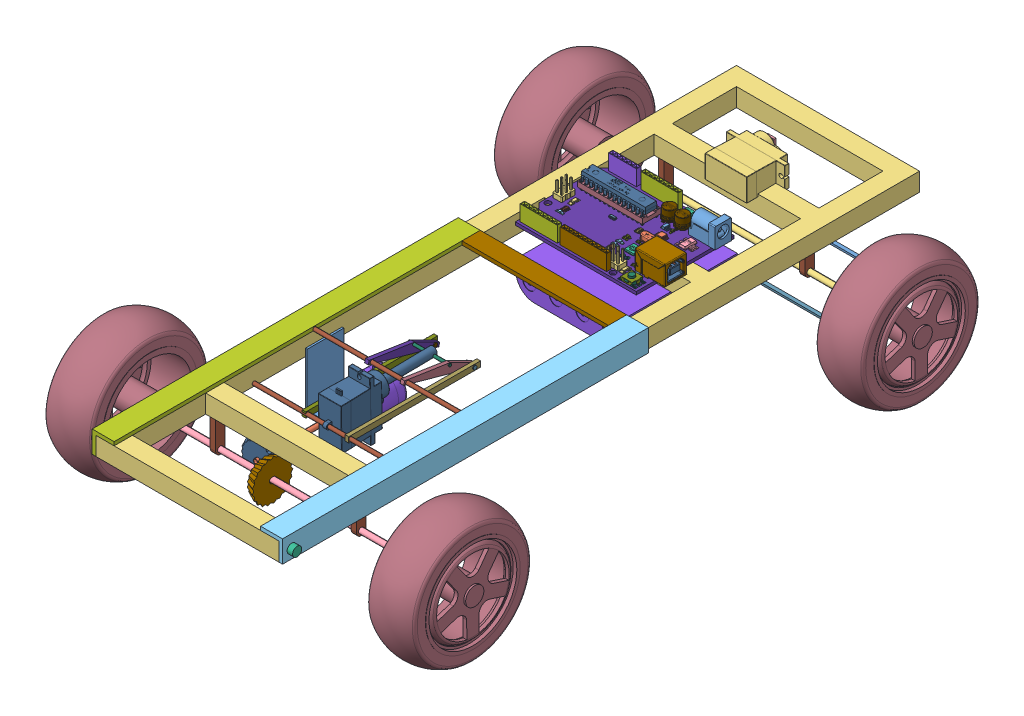
SolidWorks assembly Truck, configuration Default. Lengths in mm.
Overall size (204.96 79.96 350).
143 component instances, 76 part files, 0 mates.
Components (placement in the parent):
- truck3 v8.step-1: truck3 v8.step [Default] at origin size (204.96 79.96 350)
  - front axis.step-1: front axis.step [Default] at (0 -2.5 0) size (144 3 3)
    - Component11.step-1: Component11.step [Default] at origin size (2 2 2)
    - Component12.step-1: Component12.step [Default] at origin size (2 2 2)
    - front axis-0.step-1: front axis-0.step [Default] at origin size (140 3 3)
    - front axis-1.step-1: front axis-1.step [Default] at origin size (2 0.5 2.24)
    - front axis-2.step-1: front axis-2.step [Default] at origin size (2 0.5 2.24)
  - _Battery Holder.914559a7-a8a6-4aca-8b1f-9f589b69178d.step-1: _Battery Holder.914559a7-a8a6-4aca-8b1f-9f589b69178d.step [Default] at (0 -0.1583 -190) x (0 0 1) z (1 0 0) size (63 16 58)
    - Component1.step-1: Component1.step [Default] at origin size (13.02 9.16 9.21)
    - Component1.step-2: Component1.step [Default] at (0 0 -29) size (13.02 9.16 9.21)
    - Component2.step-1: Component2.step [Default] at origin size (13.02 9.28 9.51)
    - Component2.step-2: Component2.step [Default] at (0 0 -29) size (13.02 9.28 9.51)
    - _Battery Holder.914559a7-a8a6-4aca-8b1f-9f589b69178d-3.step-1: _Battery Holder.914559a7-a8a6-4aca-8b1f-9f589b69178d-3.step [Default] at origin size (63 16 58)
  - Arduino_uno.6df525b0-a0fc-4683-8e1a-4d70c617ad71.step-1: Arduino_uno.6df525b0-a0fc-4683-8e1a-4d70c617ad71.step [Default] at (32.62 13 -215.96) x (0 0 -1) z (1 0 0) size (53.34 15.25 74.93)
    - USB type b.step-1: USB type b.step [Default] at (-38.02 0.43 6.35) size (13.72 15.2 16.5)
      - USB SHELL.step-1: USB SHELL.step [Default] at origin size (13.72 15.2 16.5)
      - USB core.step-1: USB core.step [Default] at origin size (11.3 10.68 15.75)
      - usb top contact.step-1: usb top contact.step [Default] at (1.25 6.09 -0.38) size (1 9.67 13.76)
      - usb btm contact.step-1: usb btm contact.step [Default] at (1.25 4.41 -0.38) size (1 6.84 11.76)
      - usb btm contact.step-2: usb btm contact.step [Default] at (-1.25 4.41 -0.38) size (1 6.84 11.76)
      - usb top contact.step-2: usb top contact.step [Default] at (-1.25 6.09 -0.38) size (1 9.67 13.76)
    - dip28 (1).step-1: dip28 (1).step [Default] at (-16.383 1.5 -46.355) x (0 0 -1) z (1 0 0) size (35.48 7.37 10.1)
      - dip28.step-1: dip28.step [Default] at origin size (35.48 2.8 10.1)
      - dip socket pin.step-1: dip socket pin.step [Default] at (16.51 2.8 -3.81) size (1.7 7.37 1.7)
      - dip socket pin.step-2: dip socket pin.step [Default] at (16.51 2.8 3.81) size (1.7 7.37 1.7)
      - dip socket pin.step-3: dip socket pin.step [Default] at (13.97 2.8 -3.81) size (1.7 7.37 1.7)
      - dip socket pin.step-4: dip socket pin.step [Default] at (13.97 2.8 3.81) size (1.7 7.37 1.7)
      - dip socket pin.step-5: dip socket pin.step [Default] at (11.43 2.8 -3.81) size (1.7 7.37 1.7)
      - dip socket pin.step-6: dip socket pin.step [Default] at (11.43 2.8 3.81) size (1.7 7.37 1.7)
      - dip socket pin.step-7: dip socket pin.step [Default] at (8.89 2.8 -3.81) size (1.7 7.37 1.7)
      - dip socket pin.step-8: dip socket pin.step [Default] at (8.89 2.8 3.81) size (1.7 7.37 1.7)
      - dip socket pin.step-9: dip socket pin.step [Default] at (6.35 2.8 -3.81) size (1.7 7.37 1.7)
      - dip socket pin.step-10: dip socket pin.step [Default] at (6.35 2.8 3.81) size (1.7 7.37 1.7)
      - dip socket pin.step-11: dip socket pin.step [Default] at (3.81 2.8 -3.81) size (1.7 7.37 1.7)
      - dip socket pin.step-12: dip socket pin.step [Default] at (3.81 2.8 3.81) size (1.7 7.37 1.7)
      - dip socket pin.step-13: dip socket pin.step [Default] at (1.27 2.8 -3.81) size (1.7 7.37 1.7)
      - dip socket pin.step-14: dip socket pin.step [Default] at (1.27 2.8 3.81) size (1.7 7.37 1.7)
      - dip socket pin.step-15: dip socket pin.step [Default] at (-1.27 2.8 -3.81) size (1.7 7.37 1.7)
      - dip socket pin.step-16: dip socket pin.step [Default] at (-1.27 2.8 3.81) size (1.7 7.37 1.7)
      - dip socket pin.step-17: dip socket pin.step [Default] at (-3.81 2.8 -3.81) size (1.7 7.37 1.7)
      - dip socket pin.step-18: dip socket pin.step [Default] at (-3.81 2.8 3.81) size (1.7 7.37 1.7)
      - dip socket pin.step-19: dip socket pin.step [Default] at (-6.35 2.8 -3.81) size (1.7 7.37 1.7)
      - dip socket pin.step-20: dip socket pin.step [Default] at (-6.35 2.8 3.81) size (1.7 7.37 1.7)
      - dip socket pin.step-21: dip socket pin.step [Default] at (-8.89 2.8 -3.81) size (1.7 7.37 1.7)
      - dip socket pin.step-22: dip socket pin.step [Default] at (-8.89 2.8 3.81) size (1.7 7.37 1.7)
      - dip socket pin.step-23: dip socket pin.step [Default] at (-11.43 2.8 -3.81) size (1.7 7.37 1.7)
      - dip socket pin.step-24: dip socket pin.step [Default] at (-11.43 2.8 3.81) size (1.7 7.37 1.7)
      - dip socket pin.step-25: dip socket pin.step [Default] at (-13.97 2.8 -3.81) size (1.7 7.37 1.7)
      - dip socket pin.step-26: dip socket pin.step [Default] at (-13.97 2.8 3.81) size (1.7 7.37 1.7)
      - dip socket pin.step-27: dip socket pin.step [Default] at (-16.51 2.8 -3.81) size (1.7 7.37 1.7)
      - dip socket pin.step-28: dip socket pin.step [Default] at (-16.51 2.8 3.81) size (1.7 7.37 1.7)
    - RESET BUTTON.step-1: RESET BUTTON.step [Default] at (-49.403 0 -6.35) size (6.2 3.1 9.6)
      - RESET CORE.step-1: RESET CORE.step [Default] at (0 0.1 0) x (-1 0 0) z (0 0 -1) size (6.2 3.1 9.6)
      - RESET.step-1: RESET.step [Default] at (0 0.1 0) x (0 0 1) z (-1 0 0) size (7.3 2 6.2)
    - unoboard blue.step-1: unoboard blue.step [Default] at origin size (53.34 1.65 68.58)
    - 47uf CAP Dcase.step-1: 47uf CAP Dcase.step [Default] at (-9.4141 0 -18.4991) x (0 0 -1) z (1 0 0) size (6.6 5.81 8)
    - power jack.step-1: power jack.step [Default] at (-7.675 0 1.905) size (11.2 15.2 15.9)
    - 47uf CAP Dcase.step-2: 47uf CAP Dcase.step [Default] at (-9.4141 0 -25.7132) x (0 0 -1) z (1 0 0) size (6.6 5.81 8)
    - crystal.step-1: crystal.step [Default] at (-26.162 0 -18.923) x (1 0 0) z (0 0 -1) size (4 5 11)
    - 2pin_header__02.step-1: 2pin_header__02.step [Default] at (-46.23 0 -15.75) size (5 11.75 2.54)
    - nano - reg.step-1: nano - reg.step [Default] at (-17.399 0 -7.747) size (6.5 1.69 8.3)
    - led.step-1: led.step [Default] at (-34.29 0 -27.94) x (0 0 1) z (-1 0 0) size (4 0.85 1.47)
    - 2pin_header__02.step-2: 2pin_header__02.step [Default] at (-30.43 0 -64.91) x (0 0 1) z (-1 0 0) size (5 11.75 2.54)
    - 2pin_header__02.step-3: 2pin_header__02.step [Default] at (-27.89 0 -64.91) x (0 0 1) z (-1 0 0) size (5 11.75 2.54)
    - 2pin_header__02.step-4: 2pin_header__02.step [Default] at (-25.35 0 -64.91) x (0 0 1) z (-1 0 0) size (5 11.75 2.54)
    - 2pin_header__02.step-5: 2pin_header__02.step [Default] at (-46.23 0 -18.29) size (5 11.75 2.54)
    - 2pin_header__02.step-6: 2pin_header__02.step [Default] at (-46.23 0 -20.83) size (5 11.75 2.54)
    - atmega16u2.step-1: atmega16u2.step [Default] at (-34.671 0.06 -20) x (1 0 0) z (0 0 -1) size (5.5 1.01 5.5)
    - led.step-2: led.step [Default] at (-36.83 0 -27.94) x (0 0 1) z (-1 0 0) size (4 0.85 1.47)
    - led.step-3: led.step [Default] at (-42.037 0 -27.94) x (0 0 1) z (-1 0 0) size (4 0.85 1.47)
    - led.step-4: led.step [Default] at (-36.576 0 -58.42) x (0 0 1) z (-1 0 0) size (4 0.85 1.47)
    - 8 PORT HEADER.step-1: 8 PORT HEADER.step [Default] at (-50.8 0 -45.72) x (0 0 -1) z (1 0 0) size (20.32 10.51 2.41)
    - 8 PORT HEADER.step-2: 8 PORT HEADER.step [Default] at (-2.54 0 -27.94) x (0 0 -1) z (1 0 0) size (20.32 10.51 2.41)
    - 6 PORT HEADER.step-1: 6 PORT HEADER.step [Default] at (-2.54 0 -50.8) x (0 0 -1) z (1 0 0) size (15.24 10.51 2.41)
    - 10 PORT HEADER.step-1: 10 PORT HEADER.step [Default] at (-50.8 0 -18.796) x (0 0 -1) z (1 0 0) size (25.4 10.51 2.41)
    - ATMEL328P.step-1: ATMEL328P.step [Default] at (-16.383 4.3 -46.355) x (0 0 -1) z (1 0 0) size (35 7.27 7.87)
    - 102 RESISTOR PACK.step-1: 102 RESISTOR PACK.step [Default] at (-33.782 0 -58.42) size (3.2 0.46 3)
    - 102 RESISTOR PACK.step-2: 102 RESISTOR PACK.step [Default] at (-39.37 0 -27.94) size (3.2 0.46 3)
    - 103 RESISTOR PACK.step-1: 103 RESISTOR PACK.step [Default] at (-23.876 0 -27.94) size (3.2 0.46 3)
    - 220 RESISTOR PACK.step-1: 220 RESISTOR PACK.step [Default] at (-36.83 0 -12.827) size (3.2 0.46 3)
    - 16mhz crystal - measured.step-1: 16mhz crystal - measured.step [Default] at (-24.892 0 -41.275) x (0 0 -1) z (1 0 0) size (3.4 0.8 2)
    - PADS001.step-1: PADS001.step [Default] at (-39.878 0.1 -18.288) x (-1 0 0) z (0 0 1) size (4.54 0.1 4.54)
    - 603 cap on pad.step-1: 603 cap on pad.step [Default] at (-44.45 0 -27.94) x (0 0 -1) z (1 0 0) size (2.76 0.9 1.02)
    - ssot3.step-1: ssot3.step [Default] at (-26.5 0 -8.128) x (-1 0 0) z (0 0 -1) size (3 1.13 3.09)
    - mf-msmf050-2.step-1: mf-msmf050-2.step [Default] at (-26.5 0 -4.064) size (5.83 1.02 3.72)
    - 603 cap on pad.step-2: 603 cap on pad.step [Default] at (-29.845 0 -27.94) x (0 0 -1) z (1 0 0) size (2.76 0.9 1.02)
    - 603 cap on pad.step-3: 603 cap on pad.step [Default] at (-31.496 0 -27.94) x (0 0 -1) z (1 0 0) size (2.76 0.9 1.02)
    - lmv358.step-1: lmv358.step [Default] at (-15.24 0 -21.971) x (0 0 -1) z (1 0 0) size (3.7 1.4 2.9)
    - 603 cap on pad.step-4: 603 cap on pad.step [Default] at (-15.24 0 -18.415) size (2.76 0.9 1.02)
    - 603 cap on pad.step-5: 603 cap on pad.step [Default] at (-29.845 0 -12.065) x (0 0 1) z (-1 0 0) size (2.76 0.9 1.02)
    - 603 cap on pad.step-6: 603 cap on pad.step [Default] at (-29.591 0 -22.352) x (0 0 1) z (-1 0 0) size (2.76 0.9 1.02)
    - 603 cap on pad.step-7: 603 cap on pad.step [Default] at (-29.591 0 -16.002) x (0 0 1) z (-1 0 0) size (2.76 0.9 1.02)
    - 603 cap on pad.step-8: 603 cap on pad.step [Default] at (-41.91 0 -12.7) x (0 0 1) z (-1 0 0) size (2.76 0.9 1.02)
    - lp2985dgkr.step-1: lp2985dgkr.step [Default] at (-20.32 0 -19.05) x (0 0 -1) z (1 0 0) size (5.85 1.1 3)
    - cd1206 diode.step-1: cd1206 diode.step [Default] at (-27.94 0 -59.436) x (0 0 -1) z (1 0 0) size (2 0.96 5)
    - cd1206 diode.step-2: cd1206 diode.step [Default] at (-46.228 0 -13.081) x (0 0 1) z (-1 0 0) size (2 0.96 5)
    - 603 resistor.step-1: 603 resistor.step [Default] at (-29.591 0 -19.05) x (0 0 1) z (-1 0 0) size (2.36 0.61 1.02)
    - blm21.step-1: blm21.step [Default] at (-45.085 0 -7.62) x (0 0 -1) z (1 0 0) size (2.78 0.95 1.32)
    - m7 diode.step-1: m7 diode.step [Default] at (-2.794 0 -21.59) x (0 0 -1) z (1 0 0) size (6.66 2.35 2.5)
    - MLC0603.step-1: MLC0603.step [Default] at (-33.655 0 -12.827) x (0 0 -1) z (1 0 0) size (2.36 0.6 1.02)
    - MLC0603.step-2: MLC0603.step [Default] at (-39.37 0 -12.827) x (0 0 -1) z (1 0 0) size (2.36 0.6 1.02)
  - motor.step-1: motor.step [Default] at (110 -2.6 -50) size (20 17.52 33.3)
    - DC Motor.step-1: DC Motor.step [Default] at (-131.4567 -14.8772 -31.9864) x (0 0 -1) z (1 0 0) size (33.3 17.52 20)
  - _Bryce Gear.7a5ef56f-171a-427d-9286-492b84cab965 v1.step-1: _Bryce Gear.7a5ef56f-171a-427d-9286-492b84cab965 v1.step [Default] at (4 -17.4592 -12.8991) x (1 0 0) z (0 1 0) size (24.9 22.15 22.26)
    - Component36.step-1: Component36.step [Default] at origin size (5 22.15 22.21)
    - _Bryce Gear.7a5ef56f-171a-427d-9286-492b84cab965 v1-4.step-1: _Bryce Gear.7a5ef56f-171a-427d-9286-492b84cab965 v1-4.step [Default] at origin size (22.15 5 22.21)
  - hooks.step-1: hooks.step [Default] at origin size (3 20 5)
  - hooks.step-2: hooks.step [Default] at (-77 0 0) size (3 20 5)
  - link.step-1: link.step [Default] at (10 0 0) size (2 1 40)
  - l F wheel.step-1: l F wheel.step [Default] at (66.621 -3598 -2553.8593) x (0 0 1) z (-1 0 0) size (78.1 78.1 30.8)
  - link3.step-1: link3.step [Default] at origin size (144 1 2)
  - l F wheel.step-2: l F wheel.step [Default] at (-66.1407 -3598 2054.621) x (0 0 -1) z (1 0 0) size (78.1 78.1 30.8)
  - pin.step-1: pin.step [Default] at origin size (1.5 3 1.5)
  - link2.step-1: link2.step [Default] at origin size (2 1 20)
  - pin2.step-1: pin2.step [Default] at origin size (1.5 3 1.5)
  - Component10.step-1: Component10.step [Default] at origin size (2 0.5 2)
  - Component13.step-1: Component13.step [Default] at origin size (72 1 2)
  - Component14.step-1: Component14.step [Default] at origin size (2 0.5 2)
  - Servo v1 v1 (1).step-1: Servo v1 v1 (1).step [Default] at (-6 20.6434 -255.1566) x (1 0 0) z (0 1 0) size (32.1 29.4 12.51)
  - hooks.step-3: hooks.step [Default] at (-77 0 245) size (3 20 5)
  - hooks.step-4: hooks.step [Default] at (0 0 245) size (3 20 5)
  - axis2.step-1: axis2.step [Default] at (0 0 45) size (144 3 3)
  - l F wheel.step-3: l F wheel.step [Default] at (66.621 -3598 -2308.8593) x (0 0 1) z (-1 0 0) size (78.1 78.1 30.8)
  - l F wheel.step-4: l F wheel.step [Default] at (-66.1407 -3598 2299.621) x (0 0 -1) z (1 0 0) size (78.1 78.1 30.8)
  - truck bed chassis.step-1: truck bed chassis.step [Default] at (0 0 50) size (12 12 200)
  - TRUCK BED PIN.step-1: TRUCK BED PIN.step [Default] at (0 0 50) size (3 5 5)
  - truck bed chassis(Mirror).step-1: truck bed chassis(Mirror).step [Default] at (0 0 50) x (-1 0 0) z (0 0 -1) size (12 12 200)
  - TRUCK BED PIN(Mirror).step-1: TRUCK BED PIN(Mirror).step [Default] at (0 0 50) x (-1 0 0) z (0 0 -1) size (3 5 5)
  - Component20.step-1: Component20.step [Default] at (0 0 50) size (80 2 10)
  - Servo v1 v1.step-1: Servo v1 v1.step [Default] at (5.9799 13.1118 -43.8375) x (0 -0.999848 -0.017452) z (1 0 0) size (32.1 59.4 12.51)
  - Component23.step-1: Component23.step [Default] at (0.1067 -4.9119 40.1201) size (80 2 2)
  - Component26.step-1: Component26.step [Default] at (5.3633 11.3025 0.111) x (0 -1 0.000933) z (0 0.000933 1) size (3 2 72)
  - Component27.step-1: Component27.step [Default] at (8.7 -20.5871 -74.9158) x (1 0 0) z (0 0.267238 0.96363) size (2 5 40)
  - Component28.step-1: Component28.step [Default] at (0 20.7193 -0.8092) x (1 0 0) z (0 0.267238 0.96363) size (5 2 2)
  - Component23.step-2: Component23.step [Default] at (0 4.1 6.9) size (80 2 2)
  - Component29.step-1: Component29.step [Default] at origin size (22.5 1.5 1.5)
  - Component26(Mirror).step-1: Component26(Mirror).step [Default] at (-5.2566 11.1898 0) x (0 -1 0) z (0 0 -1) size (3 2 72)
  - Component27(Mirror).step-1: Component27(Mirror).step [Default] at (-8.7 -20.5871 -74.9158) x (-1 0 0) z (0 -0.267238 -0.96363) size (2 5 40)
  - Component28(Mirror).step-1: Component28(Mirror).step [Default] at (0 20.7193 -0.8092) x (-1 0 0) z (0 -0.267238 -0.96363) size (5 2 2)
  - Component37.step-1: Component37.step [Default] at (-39.9847 -101 -74.4847) x (0 0 1) z (-1 0 0) size (20 30 27)
  - Component38.step-1: Component38.step [Default] at (-4 0 0) size (2.5 2.5 43)
  - truck3.step-1: truck3.step [Default] at origin size (100 10 350)
  - truck3-5.step-1: truck3-5.step [Default] at origin size (4.6 33.04 1)
